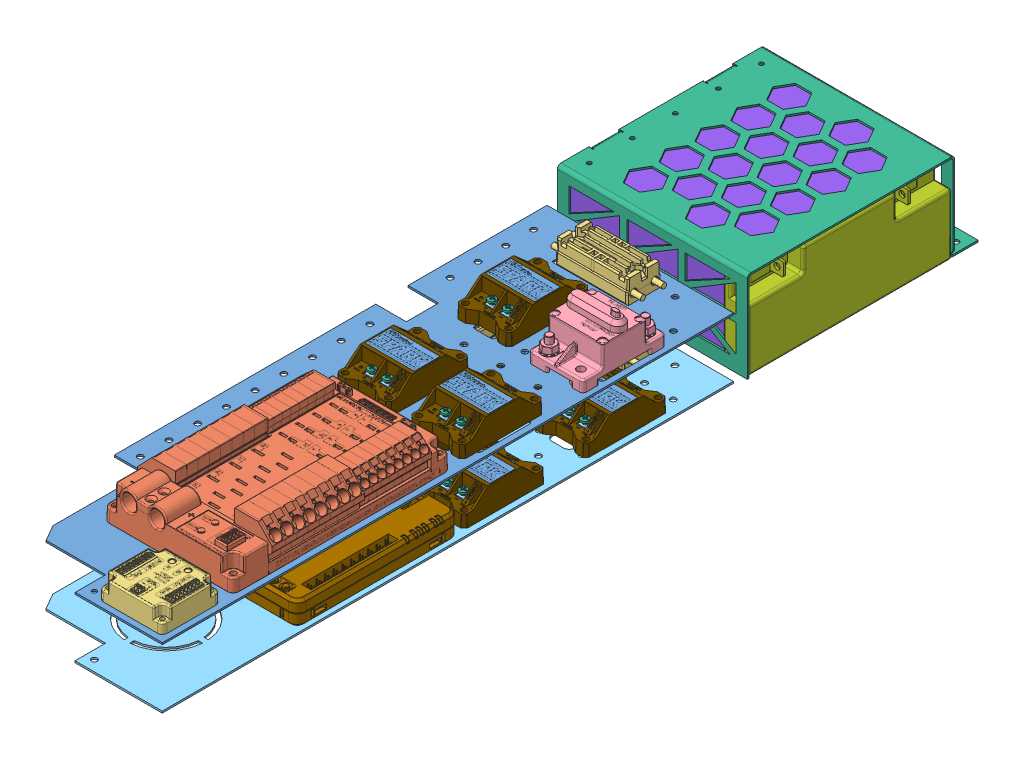
SolidWorks assembly 0001 - 05 - 1000 ELECTRONICS BOARD, configuration Default. Lengths in mm.
Overall size (954.35 3032.57 828.17).
277 component instances, 28 part files, 29 mates.
Components (placement in the parent):
- 0001 - 05 - 0001 Reference Geometry-1: 0001 - 05 - 0001 Reference Geometry [Default] at origin size (945.82 0 799.08) (hidden)
- 0001 - 05 - 1010 ELECTRONICS BOARD BOTTOM-1: 0001 - 05 - 1010 ELECTRONICS BOARD BOTTOM [Default] at (8.5296 2988.8325 -29.0866) size (945.82 43.74 799.08)
  - 0001 - 05 - 0001 Reference Geometry-1: 0001 - 05 - 0001 Reference Geometry [Default] at origin size (945.82 0 799.08) (hidden)
  - 0001 - 05 - 1011 Bottom Board-1: 0001 - 05 - 1011 Bottom Board [Default] at origin size (165.1 1.59 505.59)
  - PDP_asmb-2: PDP_asmb [Default] at (-272.032 8.2677 231.0895) x (0 0 -1) z (1 0 0) size (192.68 36.15 120.93)
  - VRM-3: VRM [Default] at (-242.2924 8.7189 366.7652) size (56.39 19.92 51.56)
  - REV_SPARK-1: REV_SPARK [Default] at (-290.8098 -27.4428 120.6986) x (0 0 -1) z (1 0 0) size (73.01 22.15 47.86)
    - RR-SPARK-BD-B-Assembly-1: RR-SPARK-BD-B-Assembly [Default] at (2.3249 6.4587 12.2534) size (55.12 17.9 42.42)
      - RR-SPARK-BD-B-1: RR-SPARK-BD-B [Default] at (27.8945 25.8332 38.0904) size (53.34 3.8 40.64)
      - ScrewTerminalAssembly-1: ScrewTerminalAssembly [Default] at (15.7541 22.7195 39.4261) x (0 0 1) z (-1 0 0) size (7.87 11.69 7.87)
        - ScrewTerminalBase-1: ScrewTerminalBase [Default] at (3.4868 6.6312 8.3972) size (7.87 7.68 7.87)
        - ScrewTerminalScrew-1: ScrewTerminalScrew [Default] at (3.5041 -1.1314 8.5263) x (0.998152 0 -0.060771) z (0.060771 0 0.998152) size (7.16 8.3 7.16)
      - ScrewTerminalAssembly-2: ScrewTerminalAssembly [Default] at (56.3941 22.7195 39.4261) x (0 0 1) z (-1 0 0) size (7.87 11.69 7.87)
        - ScrewTerminalBase-1: ScrewTerminalBase [Default] at (3.4868 6.6312 8.3972) size (7.87 7.68 7.87)
        - ScrewTerminalScrew-1: ScrewTerminalScrew [Default] at (3.5041 -1.1314 8.5263) x (0.998152 0 -0.060771) z (0.060771 0 0.998152) size (7.16 8.3 7.16)
      - ScrewTerminalAssembly-3: ScrewTerminalAssembly [Default] at (15.7541 22.7195 25.4561) x (0 0 1) z (-1 0 0) size (7.87 11.69 7.87)
        - ScrewTerminalBase-1: ScrewTerminalBase [Default] at (3.4868 6.6312 8.3972) size (7.87 7.68 7.87)
        - ScrewTerminalScrew-1: ScrewTerminalScrew [Default] at (3.5041 -1.1314 8.5263) x (0.998152 0 -0.060771) z (0.060771 0 0.998152) size (7.16 8.3 7.16)
      - ScrewTerminalAssembly-4: ScrewTerminalAssembly [Default] at (56.3941 22.7195 25.4561) x (0 0 1) z (-1 0 0) size (7.87 11.69 7.87)
        - ScrewTerminalBase-1: ScrewTerminalBase [Default] at (3.4868 6.6312 8.3972) size (7.87 7.68 7.87)
        - ScrewTerminalScrew-1: ScrewTerminalScrew [Default] at (3.5041 -1.1314 8.5263) x (0.998152 0 -0.060771) z (0.060771 0 0.998152) size (7.16 8.3 7.16)
      - Header-Female-1x3-PPTC031LFBN-RC-1: Header-Female-1x3-PPTC031LFBN-RC [Default] at (7.5745 27.4332 53.3304) size (8.13 11.71 2.54)
      - Header-Female-1x3-PPTC031LFBN-RC-2: Header-Female-1x3-PPTC031LFBN-RC [Default] at (48.2145 27.4332 53.3304) size (8.13 11.71 2.54)
      - Header-Female-1x3-PPTC031LFBN-RC-3: Header-Female-1x3-PPTC031LFBN-RC [Default] at (48.2145 27.4332 55.8704) size (8.13 11.71 2.54)
      - LED-RGB-ThroughHole-1: LED-RGB-ThroughHole [Default] at (48.2145 27.4332 21.5804) x (-1 0 0) z (0 0 -1) size (5.45 12.2 5.9)
      - MOSFET-PSMN1R0-30YLC115-1: MOSFET-PSMN1R0-30YLC115 [Default] at (35.6415 27.4332 27.2954) x (0 0 -1) z (1 0 0) size (5 1.2 6.72)
      - MOSFET-PSMN1R0-30YLC115-2: MOSFET-PSMN1R0-30YLC115 [Default] at (36.5305 27.4332 33.6454) size (5 1.2 6.72)
      - MOSFET-PSMN1R0-30YLC115-3: MOSFET-PSMN1R0-30YLC115 [Default] at (36.5305 27.4332 42.5354) x (-1 0 0) z (0 0 -1) size (5 1.2 6.72)
      - MOSFET-PSMN1R0-30YLC115-4: MOSFET-PSMN1R0-30YLC115 [Default] at (35.6415 27.4332 48.8854) x (0 0 -1) z (1 0 0) size (5 1.2 6.72)
      - Varistor-1: Varistor [Default] at (52.6595 27.4332 22.5964) x (0 0 1) z (-1 0 0) size (3.4 1.02 1.45)
      - Varistor-2: Varistor [Default] at (41.2295 27.4332 53.7114) x (0 0 1) z (-1 0 0) size (3.4 1.02 1.45)
      - Crystal-1: Crystal [Default] at (17.9885 27.4332 48.3774) x (0 0 1) z (-1 0 0) size (5.2 1.5 3.4)
      - Button-PTS645SM43SMTR92LFS-1: Button-PTS645SM43SMTR92LFS [Default] at (8.0825 27.4332 21.5804) size (9 4.3 6)
      - OptoIsolator-TLP118-1: OptoIsolator-TLP118 [Default] at (14.1785 27.4332 50.4094) x (0 0 -1) z (1 0 0) size (7.02 2.2 3.7)
      - GateDriver-A4940KLPTR-T-1: GateDriver-A4940KLPTR-T [Default] at (30.1805 25.8332 53.9654) x (0 0 -1) z (-1 0 0) size (7.8 1.2 6.43)
      - MCU-PIC16F1828-I-GZ-1: MCU-PIC16F1828-I-GZ [Default] at (19.0045 25.8332 52.8224) x (-1 0 0) z (0 0 1) size (4 0.55 4)
      - Capacitor-UCL1V471MNL1GS-1: Capacitor-UCL1V471MNL1GS [Default] at (25.8625 27.4332 46.5994) x (0 0 1) z (-1 0 0) size (10.5 14.3 11.5)
      - Capacitor-UCL1V471MNL1GS-2: Capacitor-UCL1V471MNL1GS [Default] at (25.8625 27.4332 25.2634) x (0 0 1) z (-1 0 0) size (10.5 14.3 11.5)
      - Capacitor-UCL1V471MNL1GS-3: Capacitor-UCL1V471MNL1GS [Default] at (25.8625 27.4332 35.9314) x (0 0 -1) z (1 0 0) size (10.5 14.3 11.5)
      - 1mmborder-1: 1mmborder [Default] at (27.8945 25.8332 38.0904) size (55.12 1.6 42.42)
    - Spark_P01-REV-41_TOPSHELL-1: Spark_P01-REV-41_TOPSHELL [Default] at (30.1178 29.0303 87.4264) x (1 0 0) z (0 1 0) size (73.01 47.86 22.14)
    - heatsink-1: heatsink [Default] at (29.9048 43.475 28.4732) size (25.78 15.4 43.69)
    - Spark_P01-REV-41_bottom_cover-1: Spark_P01-REV-41_bottom_cover [Default] at (30.1178 29.0303 87.4264) x (1 0 0) z (0 -1 0) size (65.7 43.71 2.65)
  - REV_SPARK-2: REV_SPARK [Default] at (-356.1591 -27.4428 120.6986) x (0 0 -1) z (1 0 0) size (73.01 22.15 47.86)
    - RR-SPARK-BD-B-Assembly-1: RR-SPARK-BD-B-Assembly [Default] at (2.3249 6.4587 12.2534) size (55.12 17.9 42.42)
      - RR-SPARK-BD-B-1: RR-SPARK-BD-B [Default] at (27.8945 25.8332 38.0904) size (53.34 3.8 40.64)
      - ScrewTerminalAssembly-1: ScrewTerminalAssembly [Default] at (15.7541 22.7195 39.4261) x (0 0 1) z (-1 0 0) size (7.87 11.69 7.87)
        - ScrewTerminalBase-1: ScrewTerminalBase [Default] at (3.4868 6.6312 8.3972) size (7.87 7.68 7.87)
        - ScrewTerminalScrew-1: ScrewTerminalScrew [Default] at (3.5041 -1.1314 8.5263) x (0.998152 0 -0.060771) z (0.060771 0 0.998152) size (7.16 8.3 7.16)
      - ScrewTerminalAssembly-2: ScrewTerminalAssembly [Default] at (56.3941 22.7195 39.4261) x (0 0 1) z (-1 0 0) size (7.87 11.69 7.87)
        - ScrewTerminalBase-1: ScrewTerminalBase [Default] at (3.4868 6.6312 8.3972) size (7.87 7.68 7.87)
        - ScrewTerminalScrew-1: ScrewTerminalScrew [Default] at (3.5041 -1.1314 8.5263) x (0.998152 0 -0.060771) z (0.060771 0 0.998152) size (7.16 8.3 7.16)
      - ScrewTerminalAssembly-3: ScrewTerminalAssembly [Default] at (15.7541 22.7195 25.4561) x (0 0 1) z (-1 0 0) size (7.87 11.69 7.87)
        - ScrewTerminalBase-1: ScrewTerminalBase [Default] at (3.4868 6.6312 8.3972) size (7.87 7.68 7.87)
        - ScrewTerminalScrew-1: ScrewTerminalScrew [Default] at (3.5041 -1.1314 8.5263) x (0.998152 0 -0.060771) z (0.060771 0 0.998152) size (7.16 8.3 7.16)
      - ScrewTerminalAssembly-4: ScrewTerminalAssembly [Default] at (56.3941 22.7195 25.4561) x (0 0 1) z (-1 0 0) size (7.87 11.69 7.87)
        - ScrewTerminalBase-1: ScrewTerminalBase [Default] at (3.4868 6.6312 8.3972) size (7.87 7.68 7.87)
        - ScrewTerminalScrew-1: ScrewTerminalScrew [Default] at (3.5041 -1.1314 8.5263) x (0.998152 0 -0.060771) z (0.060771 0 0.998152) size (7.16 8.3 7.16)
      - Header-Female-1x3-PPTC031LFBN-RC-1: Header-Female-1x3-PPTC031LFBN-RC [Default] at (7.5745 27.4332 53.3304) size (8.13 11.71 2.54)
      - Header-Female-1x3-PPTC031LFBN-RC-2: Header-Female-1x3-PPTC031LFBN-RC [Default] at (48.2145 27.4332 53.3304) size (8.13 11.71 2.54)
      - Header-Female-1x3-PPTC031LFBN-RC-3: Header-Female-1x3-PPTC031LFBN-RC [Default] at (48.2145 27.4332 55.8704) size (8.13 11.71 2.54)
      - LED-RGB-ThroughHole-1: LED-RGB-ThroughHole [Default] at (48.2145 27.4332 21.5804) x (-1 0 0) z (0 0 -1) size (5.45 12.2 5.9)
      - MOSFET-PSMN1R0-30YLC115-1: MOSFET-PSMN1R0-30YLC115 [Default] at (35.6415 27.4332 27.2954) x (0 0 -1) z (1 0 0) size (5 1.2 6.72)
      - MOSFET-PSMN1R0-30YLC115-2: MOSFET-PSMN1R0-30YLC115 [Default] at (36.5305 27.4332 33.6454) size (5 1.2 6.72)
      - MOSFET-PSMN1R0-30YLC115-3: MOSFET-PSMN1R0-30YLC115 [Default] at (36.5305 27.4332 42.5354) x (-1 0 0) z (0 0 -1) size (5 1.2 6.72)
      - MOSFET-PSMN1R0-30YLC115-4: MOSFET-PSMN1R0-30YLC115 [Default] at (35.6415 27.4332 48.8854) x (0 0 -1) z (1 0 0) size (5 1.2 6.72)
      - Varistor-1: Varistor [Default] at (52.6595 27.4332 22.5964) x (0 0 1) z (-1 0 0) size (3.4 1.02 1.45)
      - Varistor-2: Varistor [Default] at (41.2295 27.4332 53.7114) x (0 0 1) z (-1 0 0) size (3.4 1.02 1.45)
      - Crystal-1: Crystal [Default] at (17.9885 27.4332 48.3774) x (0 0 1) z (-1 0 0) size (5.2 1.5 3.4)
      - Button-PTS645SM43SMTR92LFS-1: Button-PTS645SM43SMTR92LFS [Default] at (8.0825 27.4332 21.5804) size (9 4.3 6)
      - OptoIsolator-TLP118-1: OptoIsolator-TLP118 [Default] at (14.1785 27.4332 50.4094) x (0 0 -1) z (1 0 0) size (7.02 2.2 3.7)
      - GateDriver-A4940KLPTR-T-1: GateDriver-A4940KLPTR-T [Default] at (30.1805 25.8332 53.9654) x (0 0 -1) z (-1 0 0) size (7.8 1.2 6.43)
      - MCU-PIC16F1828-I-GZ-1: MCU-PIC16F1828-I-GZ [Default] at (19.0045 25.8332 52.8224) x (-1 0 0) z (0 0 1) size (4 0.55 4)
      - Capacitor-UCL1V471MNL1GS-1: Capacitor-UCL1V471MNL1GS [Default] at (25.8625 27.4332 46.5994) x (0 0 1) z (-1 0 0) size (10.5 14.3 11.5)
      - Capacitor-UCL1V471MNL1GS-2: Capacitor-UCL1V471MNL1GS [Default] at (25.8625 27.4332 25.2634) x (0 0 1) z (-1 0 0) size (10.5 14.3 11.5)
      - Capacitor-UCL1V471MNL1GS-3: Capacitor-UCL1V471MNL1GS [Default] at (25.8625 27.4332 35.9314) x (0 0 -1) z (1 0 0) size (10.5 14.3 11.5)
      - 1mmborder-1: 1mmborder [Default] at (27.8945 25.8332 38.0904) size (55.12 1.6 42.42)
    - Spark_P01-REV-41_TOPSHELL-1: Spark_P01-REV-41_TOPSHELL [Default] at (30.1178 29.0303 87.4264) x (1 0 0) z (0 1 0) size (73.01 47.86 22.14)
    - heatsink-1: heatsink [Default] at (29.9048 43.475 28.4732) size (25.78 15.4 43.69)
    - Spark_P01-REV-41_bottom_cover-1: Spark_P01-REV-41_bottom_cover [Default] at (30.1178 29.0303 87.4264) x (1 0 0) z (0 -1 0) size (65.7 43.71 2.65)
  - REV_SPARK-4: REV_SPARK [Default] at (-356.1591 -27.4428 14.1852) x (0 0 -1) z (1 0 0) size (73.01 22.15 47.86)
    - RR-SPARK-BD-B-Assembly-1: RR-SPARK-BD-B-Assembly [Default] at (2.3249 6.4587 12.2534) size (55.12 17.9 42.42)
      - RR-SPARK-BD-B-1: RR-SPARK-BD-B [Default] at (27.8945 25.8332 38.0904) size (53.34 3.8 40.64)
      - ScrewTerminalAssembly-1: ScrewTerminalAssembly [Default] at (15.7541 22.7195 39.4261) x (0 0 1) z (-1 0 0) size (7.87 11.69 7.87)
        - ScrewTerminalBase-1: ScrewTerminalBase [Default] at (3.4868 6.6312 8.3972) size (7.87 7.68 7.87)
        - ScrewTerminalScrew-1: ScrewTerminalScrew [Default] at (3.5041 -1.1314 8.5263) x (0.998152 0 -0.060771) z (0.060771 0 0.998152) size (7.16 8.3 7.16)
      - ScrewTerminalAssembly-2: ScrewTerminalAssembly [Default] at (56.3941 22.7195 39.4261) x (0 0 1) z (-1 0 0) size (7.87 11.69 7.87)
        - ScrewTerminalBase-1: ScrewTerminalBase [Default] at (3.4868 6.6312 8.3972) size (7.87 7.68 7.87)
        - ScrewTerminalScrew-1: ScrewTerminalScrew [Default] at (3.5041 -1.1314 8.5263) x (0.998152 0 -0.060771) z (0.060771 0 0.998152) size (7.16 8.3 7.16)
      - ScrewTerminalAssembly-3: ScrewTerminalAssembly [Default] at (15.7541 22.7195 25.4561) x (0 0 1) z (-1 0 0) size (7.87 11.69 7.87)
        - ScrewTerminalBase-1: ScrewTerminalBase [Default] at (3.4868 6.6312 8.3972) size (7.87 7.68 7.87)
        - ScrewTerminalScrew-1: ScrewTerminalScrew [Default] at (3.5041 -1.1314 8.5263) x (0.998152 0 -0.060771) z (0.060771 0 0.998152) size (7.16 8.3 7.16)
      - ScrewTerminalAssembly-4: ScrewTerminalAssembly [Default] at (56.3941 22.7195 25.4561) x (0 0 1) z (-1 0 0) size (7.87 11.69 7.87)
        - ScrewTerminalBase-1: ScrewTerminalBase [Default] at (3.4868 6.6312 8.3972) size (7.87 7.68 7.87)
        - ScrewTerminalScrew-1: ScrewTerminalScrew [Default] at (3.5041 -1.1314 8.5263) x (0.998152 0 -0.060771) z (0.060771 0 0.998152) size (7.16 8.3 7.16)
      - Header-Female-1x3-PPTC031LFBN-RC-1: Header-Female-1x3-PPTC031LFBN-RC [Default] at (7.5745 27.4332 53.3304) size (8.13 11.71 2.54)
      - Header-Female-1x3-PPTC031LFBN-RC-2: Header-Female-1x3-PPTC031LFBN-RC [Default] at (48.2145 27.4332 53.3304) size (8.13 11.71 2.54)
      - Header-Female-1x3-PPTC031LFBN-RC-3: Header-Female-1x3-PPTC031LFBN-RC [Default] at (48.2145 27.4332 55.8704) size (8.13 11.71 2.54)
      - LED-RGB-ThroughHole-1: LED-RGB-ThroughHole [Default] at (48.2145 27.4332 21.5804) x (-1 0 0) z (0 0 -1) size (5.45 12.2 5.9)
      - MOSFET-PSMN1R0-30YLC115-1: MOSFET-PSMN1R0-30YLC115 [Default] at (35.6415 27.4332 27.2954) x (0 0 -1) z (1 0 0) size (5 1.2 6.72)
      - MOSFET-PSMN1R0-30YLC115-2: MOSFET-PSMN1R0-30YLC115 [Default] at (36.5305 27.4332 33.6454) size (5 1.2 6.72)
      - MOSFET-PSMN1R0-30YLC115-3: MOSFET-PSMN1R0-30YLC115 [Default] at (36.5305 27.4332 42.5354) x (-1 0 0) z (0 0 -1) size (5 1.2 6.72)
      - MOSFET-PSMN1R0-30YLC115-4: MOSFET-PSMN1R0-30YLC115 [Default] at (35.6415 27.4332 48.8854) x (0 0 -1) z (1 0 0) size (5 1.2 6.72)
      - Varistor-1: Varistor [Default] at (52.6595 27.4332 22.5964) x (0 0 1) z (-1 0 0) size (3.4 1.02 1.45)
      - Varistor-2: Varistor [Default] at (41.2295 27.4332 53.7114) x (0 0 1) z (-1 0 0) size (3.4 1.02 1.45)
      - Crystal-1: Crystal [Default] at (17.9885 27.4332 48.3774) x (0 0 1) z (-1 0 0) size (5.2 1.5 3.4)
      - Button-PTS645SM43SMTR92LFS-1: Button-PTS645SM43SMTR92LFS [Default] at (8.0825 27.4332 21.5804) size (9 4.3 6)
      - OptoIsolator-TLP118-1: OptoIsolator-TLP118 [Default] at (14.1785 27.4332 50.4094) x (0 0 -1) z (1 0 0) size (7.02 2.2 3.7)
      - GateDriver-A4940KLPTR-T-1: GateDriver-A4940KLPTR-T [Default] at (30.1805 25.8332 53.9654) x (0 0 -1) z (-1 0 0) size (7.8 1.2 6.43)
      - MCU-PIC16F1828-I-GZ-1: MCU-PIC16F1828-I-GZ [Default] at (19.0045 25.8332 52.8224) x (-1 0 0) z (0 0 1) size (4 0.55 4)
      - Capacitor-UCL1V471MNL1GS-1: Capacitor-UCL1V471MNL1GS [Default] at (25.8625 27.4332 46.5994) x (0 0 1) z (-1 0 0) size (10.5 14.3 11.5)
      - Capacitor-UCL1V471MNL1GS-2: Capacitor-UCL1V471MNL1GS [Default] at (25.8625 27.4332 25.2634) x (0 0 1) z (-1 0 0) size (10.5 14.3 11.5)
      - Capacitor-UCL1V471MNL1GS-3: Capacitor-UCL1V471MNL1GS [Default] at (25.8625 27.4332 35.9314) x (0 0 -1) z (1 0 0) size (10.5 14.3 11.5)
      - 1mmborder-1: 1mmborder [Default] at (27.8945 25.8332 38.0904) size (55.12 1.6 42.42)
    - Spark_P01-REV-41_TOPSHELL-1: Spark_P01-REV-41_TOPSHELL [Default] at (30.1178 29.0303 87.4264) x (1 0 0) z (0 1 0) size (73.01 47.86 22.14)
    - heatsink-1: heatsink [Default] at (29.9048 43.475 28.4732) size (25.78 15.4 43.69)
    - Spark_P01-REV-41_bottom_cover-1: Spark_P01-REV-41_bottom_cover [Default] at (30.1178 29.0303 87.4264) x (1 0 0) z (0 -1 0) size (65.7 43.71 2.65)
  - Victor SP-1: Victor SP [Default] at (-293.3197 7.7573 -79.0575) x (0 0 -1) z (1 0 0) size (30.24 20.93 80)
  - Circuit Breaker 120A-1: Circuit Breaker 120A [Default] at (-238.125 6.4135 -14.097) x (0 0 -1) z (1 0 0) size (73.72 42.2 48.95)
- 0001 - 05 - 1020 ELECTRONICS BOARD TOP-1: 0001 - 05 - 1020 ELECTRONICS BOARD TOP [Default] at (8.5296 2936.445 -28.9482) size (945.82 1.59 799.08)
  - 0001 - 05 - 0001 Reference Geometry-1: 0001 - 05 - 0001 Reference Geometry [Default] at origin size (945.82 0 799.08) (hidden)
  - 0001 - 05 - 1021 Top Board-1: 0001 - 05 - 1021 Top Board [Default] at origin size (165.1 1.59 505.59)
- Victor SP-1: Victor SP [Default] at (-345.5648 2944.2023 -57.2769) size (30.24 20.93 80)
- Victor SP-2: Victor SP [Default] at (-287.8884 2944.2023 -108.0057) x (0 0 -1) z (1 0 0) size (30.24 20.93 80)
- 0001 - 05 - 1030 Battery Mount-1: 0001 - 05 - 1030 Battery Mount [Default] at (-366.1204 2936.445 -145.8517) size (168.28 80.33 207.33)
- Battery-1: Battery [Default] at (-358.4366 2999.2297 -178.2028) x (0 0 -1) z (1 0 0) size (181.13 75.98 166.88)
  - Electrical_Yuasa_NP18-12_Top-1: Electrical_Yuasa_NP18-12_Top [Default] at origin size (181.13 75.98 21.09)
  - Electrical_Yuasa_Np18-12_Middle-1: Electrical_Yuasa_Np18-12_Middle [Default] at (114.1139 -0.254 -6.096) size (179.58 75.44 145.8)
- REV_SPARK-1: REV_SPARK [Default] at (-280.9687 2909.0022 -16.6287) x (0 0 -1) z (1 0 0) size (73.01 22.15 47.86)
  - RR-SPARK-BD-B-Assembly-1: RR-SPARK-BD-B-Assembly [Default] at (2.3249 6.4587 12.2534) size (55.12 17.9 42.42)
    - RR-SPARK-BD-B-1: RR-SPARK-BD-B [Default] at (27.8945 25.8332 38.0904) size (53.34 3.8 40.64)
    - ScrewTerminalAssembly-1: ScrewTerminalAssembly [Default] at (15.7541 22.7195 39.4261) x (0 0 1) z (-1 0 0) size (7.87 11.69 7.87)
      - ScrewTerminalBase-1: ScrewTerminalBase [Default] at (3.4868 6.6312 8.3972) size (7.87 7.68 7.87)
      - ScrewTerminalScrew-1: ScrewTerminalScrew [Default] at (3.5041 -1.1314 8.5263) x (0.998152 0 -0.060771) z (0.060771 0 0.998152) size (7.16 8.3 7.16)
    - ScrewTerminalAssembly-2: ScrewTerminalAssembly [Default] at (56.3941 22.7195 39.4261) x (0 0 1) z (-1 0 0) size (7.87 11.69 7.87)
      - ScrewTerminalBase-1: ScrewTerminalBase [Default] at (3.4868 6.6312 8.3972) size (7.87 7.68 7.87)
      - ScrewTerminalScrew-1: ScrewTerminalScrew [Default] at (3.5041 -1.1314 8.5263) x (0.998152 0 -0.060771) z (0.060771 0 0.998152) size (7.16 8.3 7.16)
    - ScrewTerminalAssembly-3: ScrewTerminalAssembly [Default] at (15.7541 22.7195 25.4561) x (0 0 1) z (-1 0 0) size (7.87 11.69 7.87)
      - ScrewTerminalBase-1: ScrewTerminalBase [Default] at (3.4868 6.6312 8.3972) size (7.87 7.68 7.87)
      - ScrewTerminalScrew-1: ScrewTerminalScrew [Default] at (3.5041 -1.1314 8.5263) x (0.998152 0 -0.060771) z (0.060771 0 0.998152) size (7.16 8.3 7.16)
    - ScrewTerminalAssembly-4: ScrewTerminalAssembly [Default] at (56.3941 22.7195 25.4561) x (0 0 1) z (-1 0 0) size (7.87 11.69 7.87)
      - ScrewTerminalBase-1: ScrewTerminalBase [Default] at (3.4868 6.6312 8.3972) size (7.87 7.68 7.87)
      - ScrewTerminalScrew-1: ScrewTerminalScrew [Default] at (3.5041 -1.1314 8.5263) x (0.998152 0 -0.060771) z (0.060771 0 0.998152) size (7.16 8.3 7.16)
    - Header-Female-1x3-PPTC031LFBN-RC-1: Header-Female-1x3-PPTC031LFBN-RC [Default] at (7.5745 27.4332 53.3304) size (8.13 11.71 2.54)
    - Header-Female-1x3-PPTC031LFBN-RC-2: Header-Female-1x3-PPTC031LFBN-RC [Default] at (48.2145 27.4332 53.3304) size (8.13 11.71 2.54)
    - Header-Female-1x3-PPTC031LFBN-RC-3: Header-Female-1x3-PPTC031LFBN-RC [Default] at (48.2145 27.4332 55.8704) size (8.13 11.71 2.54)
    - LED-RGB-ThroughHole-1: LED-RGB-ThroughHole [Default] at (48.2145 27.4332 21.5804) x (-1 0 0) z (0 0 -1) size (5.45 12.2 5.9)
    - MOSFET-PSMN1R0-30YLC115-1: MOSFET-PSMN1R0-30YLC115 [Default] at (35.6415 27.4332 27.2954) x (0 0 -1) z (1 0 0) size (5 1.2 6.72)
    - MOSFET-PSMN1R0-30YLC115-2: MOSFET-PSMN1R0-30YLC115 [Default] at (36.5305 27.4332 33.6454) size (5 1.2 6.72)
    - MOSFET-PSMN1R0-30YLC115-3: MOSFET-PSMN1R0-30YLC115 [Default] at (36.5305 27.4332 42.5354) x (-1 0 0) z (0 0 -1) size (5 1.2 6.72)
    - MOSFET-PSMN1R0-30YLC115-4: MOSFET-PSMN1R0-30YLC115 [Default] at (35.6415 27.4332 48.8854) x (0 0 -1) z (1 0 0) size (5 1.2 6.72)
    - Varistor-1: Varistor [Default] at (52.6595 27.4332 22.5964) x (0 0 1) z (-1 0 0) size (3.4 1.02 1.45)
    - Varistor-2: Varistor [Default] at (41.2295 27.4332 53.7114) x (0 0 1) z (-1 0 0) size (3.4 1.02 1.45)
    - Crystal-1: Crystal [Default] at (17.9885 27.4332 48.3774) x (0 0 1) z (-1 0 0) size (5.2 1.5 3.4)
    - Button-PTS645SM43SMTR92LFS-1: Button-PTS645SM43SMTR92LFS [Default] at (8.0825 27.4332 21.5804) size (9 4.3 6)
    - OptoIsolator-TLP118-1: OptoIsolator-TLP118 [Default] at (14.1785 27.4332 50.4094) x (0 0 -1) z (1 0 0) size (7.02 2.2 3.7)
    - GateDriver-A4940KLPTR-T-1: GateDriver-A4940KLPTR-T [Default] at (30.1805 25.8332 53.9654) x (0 0 -1) z (-1 0 0) size (7.8 1.2 6.43)
    - MCU-PIC16F1828-I-GZ-1: MCU-PIC16F1828-I-GZ [Default] at (19.0045 25.8332 52.8224) x (-1 0 0) z (0 0 1) size (4 0.55 4)
    - Capacitor-UCL1V471MNL1GS-1: Capacitor-UCL1V471MNL1GS [Default] at (25.8625 27.4332 46.5994) x (0 0 1) z (-1 0 0) size (10.5 14.3 11.5)
    - Capacitor-UCL1V471MNL1GS-2: Capacitor-UCL1V471MNL1GS [Default] at (25.8625 27.4332 25.2634) x (0 0 1) z (-1 0 0) size (10.5 14.3 11.5)
    - Capacitor-UCL1V471MNL1GS-3: Capacitor-UCL1V471MNL1GS [Default] at (25.8625 27.4332 35.9314) x (0 0 -1) z (1 0 0) size (10.5 14.3 11.5)
    - 1mmborder-1: 1mmborder [Default] at (27.8945 25.8332 38.0904) size (55.12 1.6 42.42)
  - Spark_P01-REV-41_TOPSHELL-1: Spark_P01-REV-41_TOPSHELL [Default] at (30.1178 29.0303 87.4264) x (1 0 0) z (0 1 0) size (73.01 47.86 22.14)
  - heatsink-1: heatsink [Default] at (29.9048 43.475 28.4732) size (25.78 15.4 43.69)
  - Spark_P01-REV-41_bottom_cover-1: Spark_P01-REV-41_bottom_cover [Default] at (30.1178 29.0303 87.4264) x (1 0 0) z (0 -1 0) size (65.7 43.71 2.65)
- REV_SPARK-2: REV_SPARK [Default] at (-347.681 2909.0022 -13.2567) x (0 0 -1) z (1 0 0) size (73.01 22.15 47.86)
  - RR-SPARK-BD-B-Assembly-1: RR-SPARK-BD-B-Assembly [Default] at (2.3249 6.4587 12.2534) size (55.12 17.9 42.42)
    - RR-SPARK-BD-B-1: RR-SPARK-BD-B [Default] at (27.8945 25.8332 38.0904) size (53.34 3.8 40.64)
    - ScrewTerminalAssembly-1: ScrewTerminalAssembly [Default] at (15.7541 22.7195 39.4261) x (0 0 1) z (-1 0 0) size (7.87 11.69 7.87)
      - ScrewTerminalBase-1: ScrewTerminalBase [Default] at (3.4868 6.6312 8.3972) size (7.87 7.68 7.87)
      - ScrewTerminalScrew-1: ScrewTerminalScrew [Default] at (3.5041 -1.1314 8.5263) x (0.998152 0 -0.060771) z (0.060771 0 0.998152) size (7.16 8.3 7.16)
    - ScrewTerminalAssembly-2: ScrewTerminalAssembly [Default] at (56.3941 22.7195 39.4261) x (0 0 1) z (-1 0 0) size (7.87 11.69 7.87)
      - ScrewTerminalBase-1: ScrewTerminalBase [Default] at (3.4868 6.6312 8.3972) size (7.87 7.68 7.87)
      - ScrewTerminalScrew-1: ScrewTerminalScrew [Default] at (3.5041 -1.1314 8.5263) x (0.998152 0 -0.060771) z (0.060771 0 0.998152) size (7.16 8.3 7.16)
    - ScrewTerminalAssembly-3: ScrewTerminalAssembly [Default] at (15.7541 22.7195 25.4561) x (0 0 1) z (-1 0 0) size (7.87 11.69 7.87)
      - ScrewTerminalBase-1: ScrewTerminalBase [Default] at (3.4868 6.6312 8.3972) size (7.87 7.68 7.87)
      - ScrewTerminalScrew-1: ScrewTerminalScrew [Default] at (3.5041 -1.1314 8.5263) x (0.998152 0 -0.060771) z (0.060771 0 0.998152) size (7.16 8.3 7.16)
    - ScrewTerminalAssembly-4: ScrewTerminalAssembly [Default] at (56.3941 22.7195 25.4561) x (0 0 1) z (-1 0 0) size (7.87 11.69 7.87)
      - ScrewTerminalBase-1: ScrewTerminalBase [Default] at (3.4868 6.6312 8.3972) size (7.87 7.68 7.87)
      - ScrewTerminalScrew-1: ScrewTerminalScrew [Default] at (3.5041 -1.1314 8.5263) x (0.998152 0 -0.060771) z (0.060771 0 0.998152) size (7.16 8.3 7.16)
    - Header-Female-1x3-PPTC031LFBN-RC-1: Header-Female-1x3-PPTC031LFBN-RC [Default] at (7.5745 27.4332 53.3304) size (8.13 11.71 2.54)
    - Header-Female-1x3-PPTC031LFBN-RC-2: Header-Female-1x3-PPTC031LFBN-RC [Default] at (48.2145 27.4332 53.3304) size (8.13 11.71 2.54)
    - Header-Female-1x3-PPTC031LFBN-RC-3: Header-Female-1x3-PPTC031LFBN-RC [Default] at (48.2145 27.4332 55.8704) size (8.13 11.71 2.54)
    - LED-RGB-ThroughHole-1: LED-RGB-ThroughHole [Default] at (48.2145 27.4332 21.5804) x (-1 0 0) z (0 0 -1) size (5.45 12.2 5.9)
    - MOSFET-PSMN1R0-30YLC115-1: MOSFET-PSMN1R0-30YLC115 [Default] at (35.6415 27.4332 27.2954) x (0 0 -1) z (1 0 0) size (5 1.2 6.72)
    - MOSFET-PSMN1R0-30YLC115-2: MOSFET-PSMN1R0-30YLC115 [Default] at (36.5305 27.4332 33.6454) size (5 1.2 6.72)
    - MOSFET-PSMN1R0-30YLC115-3: MOSFET-PSMN1R0-30YLC115 [Default] at (36.5305 27.4332 42.5354) x (-1 0 0) z (0 0 -1) size (5 1.2 6.72)
    - MOSFET-PSMN1R0-30YLC115-4: MOSFET-PSMN1R0-30YLC115 [Default] at (35.6415 27.4332 48.8854) x (0 0 -1) z (1 0 0) size (5 1.2 6.72)
    - Varistor-1: Varistor [Default] at (52.6595 27.4332 22.5964) x (0 0 1) z (-1 0 0) size (3.4 1.02 1.45)
    - Varistor-2: Varistor [Default] at (41.2295 27.4332 53.7114) x (0 0 1) z (-1 0 0) size (3.4 1.02 1.45)
    - Crystal-1: Crystal [Default] at (17.9885 27.4332 48.3774) x (0 0 1) z (-1 0 0) size (5.2 1.5 3.4)
    - Button-PTS645SM43SMTR92LFS-1: Button-PTS645SM43SMTR92LFS [Default] at (8.0825 27.4332 21.5804) size (9 4.3 6)
    - OptoIsolator-TLP118-1: OptoIsolator-TLP118 [Default] at (14.1785 27.4332 50.4094) x (0 0 -1) z (1 0 0) size (7.02 2.2 3.7)
    - GateDriver-A4940KLPTR-T-1: GateDriver-A4940KLPTR-T [Default] at (30.1805 25.8332 53.9654) x (0 0 -1) z (-1 0 0) size (7.8 1.2 6.43)
    - MCU-PIC16F1828-I-GZ-1: MCU-PIC16F1828-I-GZ [Default] at (19.0045 25.8332 52.8224) x (-1 0 0) z (0 0 1) size (4 0.55 4)
    - Capacitor-UCL1V471MNL1GS-1: Capacitor-UCL1V471MNL1GS [Default] at (25.8625 27.4332 46.5994) x (0 0 1) z (-1 0 0) size (10.5 14.3 11.5)
    - Capacitor-UCL1V471MNL1GS-2: Capacitor-UCL1V471MNL1GS [Default] at (25.8625 27.4332 25.2634) x (0 0 1) z (-1 0 0) size (10.5 14.3 11.5)
    - Capacitor-UCL1V471MNL1GS-3: Capacitor-UCL1V471MNL1GS [Default] at (25.8625 27.4332 35.9314) x (0 0 -1) z (1 0 0) size (10.5 14.3 11.5)
    - 1mmborder-1: 1mmborder [Default] at (27.8945 25.8332 38.0904) size (55.12 1.6 42.42)
  - Spark_P01-REV-41_TOPSHELL-1: Spark_P01-REV-41_TOPSHELL [Default] at (30.1178 29.0303 87.4264) x (1 0 0) z (0 1 0) size (73.01 47.86 22.14)
  - heatsink-1: heatsink [Default] at (29.9048 43.475 28.4732) size (25.78 15.4 43.69)
  - Spark_P01-REV-41_bottom_cover-1: Spark_P01-REV-41_bottom_cover [Default] at (30.1178 29.0303 87.4264) x (1 0 0) z (0 -1 0) size (65.7 43.71 2.65)
- REV_SPARK-3: REV_SPARK [Default] at (-280.5742 2909.0022 91.7524) x (0 0 -1) z (1 0 0) size (73.01 22.15 47.86)
  - RR-SPARK-BD-B-Assembly-1: RR-SPARK-BD-B-Assembly [Default] at (2.3249 6.4587 12.2534) size (55.12 17.9 42.42)
    - RR-SPARK-BD-B-1: RR-SPARK-BD-B [Default] at (27.8945 25.8332 38.0904) size (53.34 3.8 40.64)
    - ScrewTerminalAssembly-1: ScrewTerminalAssembly [Default] at (15.7541 22.7195 39.4261) x (0 0 1) z (-1 0 0) size (7.87 11.69 7.87)
      - ScrewTerminalBase-1: ScrewTerminalBase [Default] at (3.4868 6.6312 8.3972) size (7.87 7.68 7.87)
      - ScrewTerminalScrew-1: ScrewTerminalScrew [Default] at (3.5041 -1.1314 8.5263) x (0.998152 0 -0.060771) z (0.060771 0 0.998152) size (7.16 8.3 7.16)
    - ScrewTerminalAssembly-2: ScrewTerminalAssembly [Default] at (56.3941 22.7195 39.4261) x (0 0 1) z (-1 0 0) size (7.87 11.69 7.87)
      - ScrewTerminalBase-1: ScrewTerminalBase [Default] at (3.4868 6.6312 8.3972) size (7.87 7.68 7.87)
      - ScrewTerminalScrew-1: ScrewTerminalScrew [Default] at (3.5041 -1.1314 8.5263) x (0.998152 0 -0.060771) z (0.060771 0 0.998152) size (7.16 8.3 7.16)
    - ScrewTerminalAssembly-3: ScrewTerminalAssembly [Default] at (15.7541 22.7195 25.4561) x (0 0 1) z (-1 0 0) size (7.87 11.69 7.87)
      - ScrewTerminalBase-1: ScrewTerminalBase [Default] at (3.4868 6.6312 8.3972) size (7.87 7.68 7.87)
      - ScrewTerminalScrew-1: ScrewTerminalScrew [Default] at (3.5041 -1.1314 8.5263) x (0.998152 0 -0.060771) z (0.060771 0 0.998152) size (7.16 8.3 7.16)
    - ScrewTerminalAssembly-4: ScrewTerminalAssembly [Default] at (56.3941 22.7195 25.4561) x (0 0 1) z (-1 0 0) size (7.87 11.69 7.87)
      - ScrewTerminalBase-1: ScrewTerminalBase [Default] at (3.4868 6.6312 8.3972) size (7.87 7.68 7.87)
      - ScrewTerminalScrew-1: ScrewTerminalScrew [Default] at (3.5041 -1.1314 8.5263) x (0.998152 0 -0.060771) z (0.060771 0 0.998152) size (7.16 8.3 7.16)
    - Header-Female-1x3-PPTC031LFBN-RC-1: Header-Female-1x3-PPTC031LFBN-RC [Default] at (7.5745 27.4332 53.3304) size (8.13 11.71 2.54)
    - Header-Female-1x3-PPTC031LFBN-RC-2: Header-Female-1x3-PPTC031LFBN-RC [Default] at (48.2145 27.4332 53.3304) size (8.13 11.71 2.54)
    - Header-Female-1x3-PPTC031LFBN-RC-3: Header-Female-1x3-PPTC031LFBN-RC [Default] at (48.2145 27.4332 55.8704) size (8.13 11.71 2.54)
    - LED-RGB-ThroughHole-1: LED-RGB-ThroughHole [Default] at (48.2145 27.4332 21.5804) x (-1 0 0) z (0 0 -1) size (5.45 12.2 5.9)
    - MOSFET-PSMN1R0-30YLC115-1: MOSFET-PSMN1R0-30YLC115 [Default] at (35.6415 27.4332 27.2954) x (0 0 -1) z (1 0 0) size (5 1.2 6.72)
    - MOSFET-PSMN1R0-30YLC115-2: MOSFET-PSMN1R0-30YLC115 [Default] at (36.5305 27.4332 33.6454) size (5 1.2 6.72)
    - MOSFET-PSMN1R0-30YLC115-3: MOSFET-PSMN1R0-30YLC115 [Default] at (36.5305 27.4332 42.5354) x (-1 0 0) z (0 0 -1) size (5 1.2 6.72)
    - MOSFET-PSMN1R0-30YLC115-4: MOSFET-PSMN1R0-30YLC115 [Default] at (35.6415 27.4332 48.8854) x (0 0 -1) z (1 0 0) size (5 1.2 6.72)
    - Varistor-1: Varistor [Default] at (52.6595 27.4332 22.5964) x (0 0 1) z (-1 0 0) size (3.4 1.02 1.45)
    - Varistor-2: Varistor [Default] at (41.2295 27.4332 53.7114) x (0 0 1) z (-1 0 0) size (3.4 1.02 1.45)
    - Crystal-1: Crystal [Default] at (17.9885 27.4332 48.3774) x (0 0 1) z (-1 0 0) size (5.2 1.5 3.4)
    - Button-PTS645SM43SMTR92LFS-1: Button-PTS645SM43SMTR92LFS [Default] at (8.0825 27.4332 21.5804) size (9 4.3 6)
    - OptoIsolator-TLP118-1: OptoIsolator-TLP118 [Default] at (14.1785 27.4332 50.4094) x (0 0 -1) z (1 0 0) size (7.02 2.2 3.7)
    - GateDriver-A4940KLPTR-T-1: GateDriver-A4940KLPTR-T [Default] at (30.1805 25.8332 53.9654) x (0 0 -1) z (-1 0 0) size (7.8 1.2 6.43)
    - MCU-PIC16F1828-I-GZ-1: MCU-PIC16F1828-I-GZ [Default] at (19.0045 25.8332 52.8224) x (-1 0 0) z (0 0 1) size (4 0.55 4)
    - Capacitor-UCL1V471MNL1GS-1: Capacitor-UCL1V471MNL1GS [Default] at (25.8625 27.4332 46.5994) x (0 0 1) z (-1 0 0) size (10.5 14.3 11.5)
    - Capacitor-UCL1V471MNL1GS-2: Capacitor-UCL1V471MNL1GS [Default] at (25.8625 27.4332 25.2634) x (0 0 1) z (-1 0 0) size (10.5 14.3 11.5)
    - Capacitor-UCL1V471MNL1GS-3: Capacitor-UCL1V471MNL1GS [Default] at (25.8625 27.4332 35.9314) x (0 0 -1) z (1 0 0) size (10.5 14.3 11.5)
    - 1mmborder-1: 1mmborder [Default] at (27.8945 25.8332 38.0904) size (55.12 1.6 42.42)
  - Spark_P01-REV-41_TOPSHELL-1: Spark_P01-REV-41_TOPSHELL [Default] at (30.1178 29.0303 87.4264) x (1 0 0) z (0 1 0) size (73.01 47.86 22.14)
  - heatsink-1: heatsink [Default] at (29.9048 43.475 28.4732) size (25.78 15.4 43.69)
  - Spark_P01-REV-41_bottom_cover-1: Spark_P01-REV-41_bottom_cover [Default] at (30.1178 29.0303 87.4264) x (1 0 0) z (0 -1 0) size (65.7 43.71 2.65)
- REV_SPARK-4: REV_SPARK [Default] at (-347.681 2909.0022 90.9269) x (0 0 -1) z (1 0 0) size (73.01 22.15 47.86)
  - RR-SPARK-BD-B-Assembly-1: RR-SPARK-BD-B-Assembly [Default] at (2.3249 6.4587 12.2534) size (55.12 17.9 42.42)
    - RR-SPARK-BD-B-1: RR-SPARK-BD-B [Default] at (27.8945 25.8332 38.0904) size (53.34 3.8 40.64)
    - ScrewTerminalAssembly-1: ScrewTerminalAssembly [Default] at (15.7541 22.7195 39.4261) x (0 0 1) z (-1 0 0) size (7.87 11.69 7.87)
      - ScrewTerminalBase-1: ScrewTerminalBase [Default] at (3.4868 6.6312 8.3972) size (7.87 7.68 7.87)
      - ScrewTerminalScrew-1: ScrewTerminalScrew [Default] at (3.5041 -1.1314 8.5263) x (0.998152 0 -0.060771) z (0.060771 0 0.998152) size (7.16 8.3 7.16)
    - ScrewTerminalAssembly-2: ScrewTerminalAssembly [Default] at (56.3941 22.7195 39.4261) x (0 0 1) z (-1 0 0) size (7.87 11.69 7.87)
      - ScrewTerminalBase-1: ScrewTerminalBase [Default] at (3.4868 6.6312 8.3972) size (7.87 7.68 7.87)
      - ScrewTerminalScrew-1: ScrewTerminalScrew [Default] at (3.5041 -1.1314 8.5263) x (0.998152 0 -0.060771) z (0.060771 0 0.998152) size (7.16 8.3 7.16)
    - ScrewTerminalAssembly-3: ScrewTerminalAssembly [Default] at (15.7541 22.7195 25.4561) x (0 0 1) z (-1 0 0) size (7.87 11.69 7.87)
      - ScrewTerminalBase-1: ScrewTerminalBase [Default] at (3.4868 6.6312 8.3972) size (7.87 7.68 7.87)
      - ScrewTerminalScrew-1: ScrewTerminalScrew [Default] at (3.5041 -1.1314 8.5263) x (0.998152 0 -0.060771) z (0.060771 0 0.998152) size (7.16 8.3 7.16)
    - ScrewTerminalAssembly-4: ScrewTerminalAssembly [Default] at (56.3941 22.7195 25.4561) x (0 0 1) z (-1 0 0) size (7.87 11.69 7.87)
      - ScrewTerminalBase-1: ScrewTerminalBase [Default] at (3.4868 6.6312 8.3972) size (7.87 7.68 7.87)
      - ScrewTerminalScrew-1: ScrewTerminalScrew [Default] at (3.5041 -1.1314 8.5263) x (0.998152 0 -0.060771) z (0.060771 0 0.998152) size (7.16 8.3 7.16)
    - Header-Female-1x3-PPTC031LFBN-RC-1: Header-Female-1x3-PPTC031LFBN-RC [Default] at (7.5745 27.4332 53.3304) size (8.13 11.71 2.54)
    - Header-Female-1x3-PPTC031LFBN-RC-2: Header-Female-1x3-PPTC031LFBN-RC [Default] at (48.2145 27.4332 53.3304) size (8.13 11.71 2.54)
    - Header-Female-1x3-PPTC031LFBN-RC-3: Header-Female-1x3-PPTC031LFBN-RC [Default] at (48.2145 27.4332 55.8704) size (8.13 11.71 2.54)
    - LED-RGB-ThroughHole-1: LED-RGB-ThroughHole [Default] at (48.2145 27.4332 21.5804) x (-1 0 0) z (0 0 -1) size (5.45 12.2 5.9)
    - MOSFET-PSMN1R0-30YLC115-1: MOSFET-PSMN1R0-30YLC115 [Default] at (35.6415 27.4332 27.2954) x (0 0 -1) z (1 0 0) size (5 1.2 6.72)
    - MOSFET-PSMN1R0-30YLC115-2: MOSFET-PSMN1R0-30YLC115 [Default] at (36.5305 27.4332 33.6454) size (5 1.2 6.72)
    - MOSFET-PSMN1R0-30YLC115-3: MOSFET-PSMN1R0-30YLC115 [Default] at (36.5305 27.4332 42.5354) x (-1 0 0) z (0 0 -1) size (5 1.2 6.72)
    - MOSFET-PSMN1R0-30YLC115-4: MOSFET-PSMN1R0-30YLC115 [Default] at (35.6415 27.4332 48.8854) x (0 0 -1) z (1 0 0) size (5 1.2 6.72)
    - Varistor-1: Varistor [Default] at (52.6595 27.4332 22.5964) x (0 0 1) z (-1 0 0) size (3.4 1.02 1.45)
    - Varistor-2: Varistor [Default] at (41.2295 27.4332 53.7114) x (0 0 1) z (-1 0 0) size (3.4 1.02 1.45)
    - Crystal-1: Crystal [Default] at (17.9885 27.4332 48.3774) x (0 0 1) z (-1 0 0) size (5.2 1.5 3.4)
    - Button-PTS645SM43SMTR92LFS-1: Button-PTS645SM43SMTR92LFS [Default] at (8.0825 27.4332 21.5804) size (9 4.3 6)
    - OptoIsolator-TLP118-1: OptoIsolator-TLP118 [Default] at (14.1785 27.4332 50.4094) x (0 0 -1) z (1 0 0) size (7.02 2.2 3.7)
    - GateDriver-A4940KLPTR-T-1: GateDriver-A4940KLPTR-T [Default] at (30.1805 25.8332 53.9654) x (0 0 -1) z (-1 0 0) size (7.8 1.2 6.43)
    - MCU-PIC16F1828-I-GZ-1: MCU-PIC16F1828-I-GZ [Default] at (19.0045 25.8332 52.8224) x (-1 0 0) z (0 0 1) size (4 0.55 4)
    - Capacitor-UCL1V471MNL1GS-1: Capacitor-UCL1V471MNL1GS [Default] at (25.8625 27.4332 46.5994) x (0 0 1) z (-1 0 0) size (10.5 14.3 11.5)
    - Capacitor-UCL1V471MNL1GS-2: Capacitor-UCL1V471MNL1GS [Default] at (25.8625 27.4332 25.2634) x (0 0 1) z (-1 0 0) size (10.5 14.3 11.5)
    - Capacitor-UCL1V471MNL1GS-3: Capacitor-UCL1V471MNL1GS [Default] at (25.8625 27.4332 35.9314) x (0 0 -1) z (1 0 0) size (10.5 14.3 11.5)
    - 1mmborder-1: 1mmborder [Default] at (27.8945 25.8332 38.0904) size (55.12 1.6 42.42)
  - Spark_P01-REV-41_TOPSHELL-1: Spark_P01-REV-41_TOPSHELL [Default] at (30.1178 29.0303 87.4264) x (1 0 0) z (0 1 0) size (73.01 47.86 22.14)
  - heatsink-1: heatsink [Default] at (29.9048 43.475 28.4732) size (25.78 15.4 43.69)
  - Spark_P01-REV-41_bottom_cover-1: Spark_P01-REV-41_bottom_cover [Default] at (30.1178 29.0303 87.4264) x (1 0 0) z (0 -1 0) size (65.7 43.71 2.65)
- RoboRIO-1: RoboRIO [Default] at (-276.1986 2947.6845 177.4197) x (1 0 0) z (0 1 0) size (146.27 143.19 34.5)
Mates (geometry in assembly coordinates):
- Coincident1: coordinate: point of 0001 - 05 - 0001 Reference Geometry-1; point of assembly
- Concentric2: concentric aligned: cylinder of 0001 - 05 - 1010 ELECTRONICS BOARD BOTTOM-1/0001 - 05 - 1011 Bottom Board-1 through (-353.4204 2988.8325 237.5613) axis (0 1 0) radius 2.54; cylinder of 0001 - 05 - 1020 ELECTRONICS BOARD TOP-1/0001 - 05 - 1021 Top Board-1 through (-353.4204 2938.0325 237.5613) axis (0 1 0) radius 2.54
- Concentric3: concentric aligned: cylinder of 0001 - 05 - 1010 ELECTRONICS BOARD BOTTOM-1/0001 - 05 - 1011 Bottom Board-1 through (-353.4204 2988.8325 34.3613) axis (0 1 0) radius 2.54; cylinder of 0001 - 05 - 1020 ELECTRONICS BOARD TOP-1/0001 - 05 - 1021 Top Board-1 through (-353.4204 2938.0325 34.3613) axis (0 1 0) radius 2.54
- Distance1: distance = 50.8 mm anti-aligned: plane of 0001 - 05 - 1020 ELECTRONICS BOARD TOP-1/0001 - 05 - 1021 Top Board-1 through (8.5296 2938.0325 -28.9482) normal (0 1 0); plane of 0001 - 05 - 1010 ELECTRONICS BOARD BOTTOM-1/0001 - 05 - 1011 Bottom Board-1 through (8.5296 2988.8325 -29.0866) normal (0 -1 0)
- Concentric4: concentric aligned: cylinder of 0001 - 05 - 1020 ELECTRONICS BOARD TOP-1/0001 - 05 - 1021 Top Board-1 through (-313.2884 2938.0325 -108.0057) axis (0 1 0) radius 2.413; cylinder of Victor SP-2 through (-313.2884 2938.0325 -108.0057) axis (0 1 0) radius 2.413
- Coincident2: coincident anti-aligned: plane of 0001 - 05 - 1020 ELECTRONICS BOARD TOP-1/0001 - 05 - 1021 Top Board-1 through (8.5296 2938.0325 -28.9482) normal (0 1 0); plane of Victor SP-2 through (-256.1384 2938.0325 -123.1387) normal (0 -1 0)
- Parallel1: parallel aligned: line of 0001 - 05 - 1020 ELECTRONICS BOARD TOP-1/0001 - 05 - 1021 Top Board-1 through (-320.9084 2938.0325 -122.2932) axis (1 0 0); line of Victor SP-2 through (-319.5354 2938.0781 -122.1683) axis (1 0 0)
- Concentric8: concentric aligned: cylinder of 0001 - 05 - 1020 ELECTRONICS BOARD TOP-1/0001 - 05 - 1021 Top Board-1 through (-345.5648 2938.0325 -82.6769) axis (0 1 0) radius 2.413; cylinder of Victor SP-1 through (-345.5648 2938.0325 -82.6769) axis (0 1 0) radius 2.413
- Coincident5: coincident anti-aligned: plane of 0001 - 05 - 1020 ELECTRONICS BOARD TOP-1/0001 - 05 - 1021 Top Board-1 through (8.5296 2938.0325 -28.9482) normal (0 1 0); plane of Victor SP-1 through (-330.4318 2938.0325 -25.5269) normal (0 -1 0)
- Parallel4: parallel anti-aligned: line of 0001 - 05 - 1020 ELECTRONICS BOARD TOP-1/0001 - 05 - 1021 Top Board-1 through (-359.9158 2938.0325 -90.2969) axis (0 0 1); line of Victor SP-1 through (-359.7274 2938.0781 -25.6299) axis (0 0 -1)
- Coincident7: coincident aligned: plane of 0001 - 05 - 1010 ELECTRONICS BOARD BOTTOM-1/0001 - 05 - 1011 Bottom Board-1 through (-366.1204 2990.42 -12.1321) normal (-1 0 0); plane of 0001 - 05 - 1030 Battery Mount-1 through (-366.1204 3013.5975 -324.6042) normal (-1 0 0)
- Coincident8: coincident aligned: plane of 0001 - 05 - 1020 ELECTRONICS BOARD TOP-1/0001 - 05 - 1021 Top Board-1 through (8.5296 2936.445 -28.9482) normal (0 -1 0); plane of 0001 - 05 - 1030 Battery Mount-1 through (-197.8454 2936.445 -145.8517) normal (0 -1 0)
- Distance2: distance = 9.271 mm anti-aligned: plane of 0001 - 05 - 1030 Battery Mount-1 through (-197.8454 2936.445 -144.2642) normal (0 0 1); plane of 0001 - 05 - 1020 ELECTRONICS BOARD TOP-1/0001 - 05 - 1021 Top Board-1 through (8.5296 2938.0325 -134.9932) normal (0 0 -1)
- Coincident11: coincident anti-aligned: plane of 0001 - 05 - 1020 ELECTRONICS BOARD TOP-1/0001 - 05 - 1021 Top Board-1 through (8.5296 2938.0325 -28.9482) normal (0 1 0); plane of Battery-1/Electrical_Yuasa_Np18-12_Middle-1 through (-364.5326 2938.0325 -325.4297) normal (0 -1 0)
- Coincident12: coincident anti-aligned: plane of 0001 - 05 - 1030 Battery Mount-1 through (-364.5326 2936.445 -145.8517) normal (1 0 0); plane of Battery-1/Electrical_Yuasa_Np18-12_Middle-1 through (-364.5326 2975.7515 -235.6407) normal (-1 0 0)
- Coincident13: coincident anti-aligned: plane of 0001 - 05 - 1030 Battery Mount-1 through (-197.8454 2936.445 -145.8517) normal (0 0 -1); plane of Battery-1/Electrical_Yuasa_Np18-12_Middle-1 through (-364.5326 2938.0325 -145.8517) normal (0 0 1)
- Concentric9: concentric anti-aligned: cylinder of 0001 - 05 - 1020 ELECTRONICS BOARD TOP-1/0001 - 05 - 1021 Top Board-1 through (-211.397 2938.0325 -78.6552) axis (0 1 0) radius 2.54; cylinder of REV_SPARK-1/Spark_P01-REV-41_TOPSHELL-1 through (-211.397 2948.69 -78.6552) axis (0 -1 0) radius 2.5527
- Coincident14: coincident anti-aligned: plane of 0001 - 05 - 1020 ELECTRONICS BOARD TOP-1/0001 - 05 - 1021 Top Board-1 through (8.5296 2938.0325 -28.9482) normal (0 1 0); plane of REV_SPARK-1/Spark_P01-REV-41_TOPSHELL-1 through (-230.6402 2938.0325 -46.7153) normal (0 -1 0)
- Parallel5: parallel anti-aligned: line of 0001 - 05 - 1020 ELECTRONICS BOARD TOP-1/0001 - 05 - 1021 Top Board-1 through (-201.0204 2938.0325 -134.9932) axis (0 0 1); line of REV_SPARK-1/Spark_P01-REV-41_TOPSHELL-1 through (-206.6112 2938.0325 -13.1113) axis (0 0 -1)
- Concentric10: concentric anti-aligned: cylinder of 0001 - 05 - 1020 ELECTRONICS BOARD TOP-1/0001 - 05 - 1021 Top Board-1 through (-211.0026 2938.0325 29.7258) axis (0 1 0) radius 2.54; cylinder of REV_SPARK-3/Spark_P01-REV-41_TOPSHELL-1 through (-211.0026 2948.69 29.7258) axis (0 -1 0) radius 2.5527
- Coincident16: coincident anti-aligned: plane of 0001 - 05 - 1020 ELECTRONICS BOARD TOP-1/0001 - 05 - 1021 Top Board-1 through (8.5296 2938.0325 -28.9482) normal (0 1 0); plane of REV_SPARK-3/Spark_P01-REV-41_TOPSHELL-1 through (-230.2458 2938.0325 61.6657) normal (0 -1 0)
- Parallel6: parallel anti-aligned: line of 0001 - 05 - 1020 ELECTRONICS BOARD TOP-1/0001 - 05 - 1021 Top Board-1 through (-201.0204 2938.0325 -134.9932) axis (0 0 1); line of REV_SPARK-3/Spark_P01-REV-41_TOPSHELL-1 through (-206.2168 2938.0325 95.2698) axis (0 0 -1)
- Concentric11: concentric anti-aligned: circle of 0001 - 05 - 1020 ELECTRONICS BOARD TOP-1/0001 - 05 - 1021 Top Board-1; cylinder of REV_SPARK-4/Spark_P01-REV-41_TOPSHELL-1 through (-278.1094 2948.69 92.7178) axis (0 -1 0) radius 2.5527
- Coincident18: coincident anti-aligned: plane of 0001 - 05 - 1020 ELECTRONICS BOARD TOP-1/0001 - 05 - 1021 Top Board-1 through (8.5296 2938.0325 -28.9482) normal (0 1 0); plane of REV_SPARK-4/Spark_P01-REV-41_TOPSHELL-1 through (-297.3526 2938.0325 60.8402) normal (0 -1 0)
- Parallel7: parallel anti-aligned: line of 0001 - 05 - 1020 ELECTRONICS BOARD TOP-1/0001 - 05 - 1021 Top Board-1 through (-366.1204 2938.0325 247.9981) axis (0 0 -1); line of REV_SPARK-4/Spark_P01-REV-41_TOPSHELL-1 through (-321.1857 2938.0325 27.1739) axis (0 0 1)
- Concentric12: concentric anti-aligned: cylinder of 0001 - 05 - 1020 ELECTRONICS BOARD TOP-1/0001 - 05 - 1021 Top Board-1 through (-278.1094 2938.0325 -11.4657) axis (0 1 0) radius 2.54; cylinder of REV_SPARK-2/Spark_P01-REV-41_TOPSHELL-1 through (-278.1094 2948.69 -11.4657) axis (0 -1 0) radius 2.5527
- Coincident20: coincident anti-aligned: plane of 0001 - 05 - 1020 ELECTRONICS BOARD TOP-1/0001 - 05 - 1021 Top Board-1 through (8.5296 2938.0325 -28.9482) normal (0 1 0); plane of REV_SPARK-2/Spark_P01-REV-41_TOPSHELL-1 through (-297.3526 2938.0325 -43.3433) normal (0 -1 0)
- Parallel8: parallel aligned: line of 0001 - 05 - 1020 ELECTRONICS BOARD TOP-1/0001 - 05 - 1021 Top Board-1 through (-321.0682 2938.0325 -64.6874) axis (0 0 1); line of REV_SPARK-2/Spark_P01-REV-41_TOPSHELL-1 through (-321.1857 2938.0325 -77.0097) axis (0 0 1)
- Coincident22: coincident anti-aligned: plane of 0001 - 05 - 1020 ELECTRONICS BOARD TOP-1/0001 - 05 - 1021 Top Board-1 through (8.5296 2938.0325 -28.9482) normal (0 1 0); plane of RoboRIO-1 through (-276.1986 2938.0325 177.4197) normal (0 -1 0)
